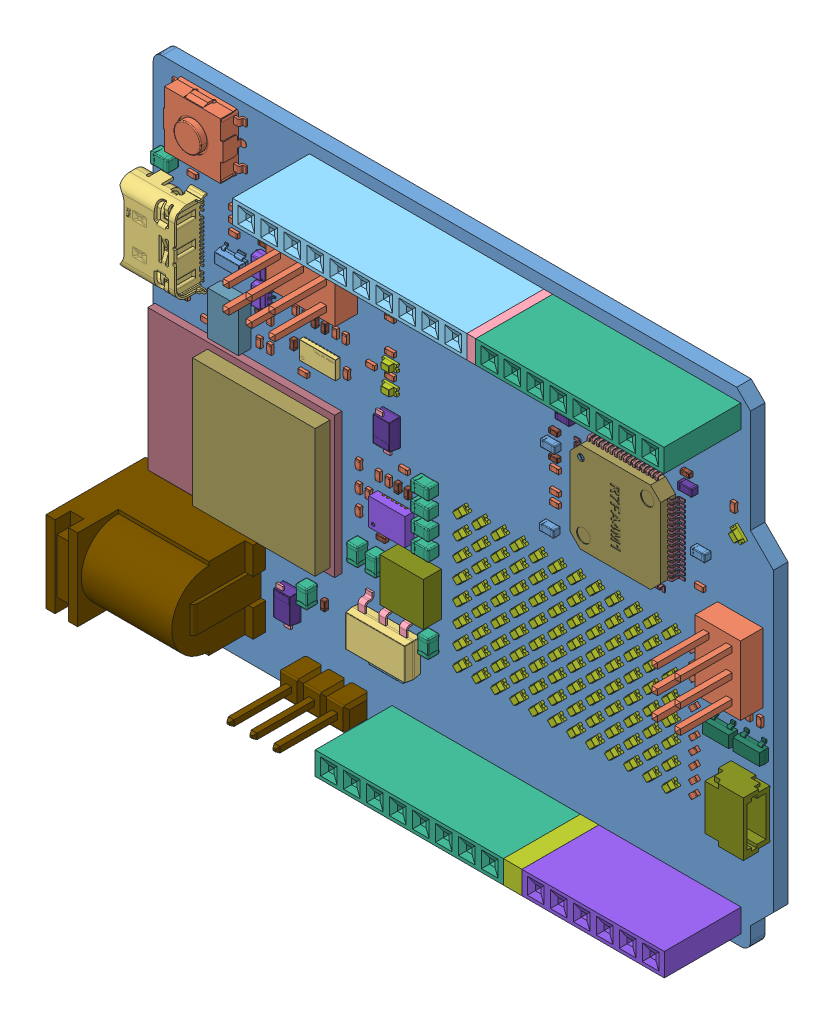
SolidWorks assembly Arduino UnoR4 Wifi PCB(ABX00087), configuration Standard. Lengths in mm.
Overall size (70.54 53.34 14.5).
574 component instances, 44 part files, 0 mates.
Components (placement in the parent):
- PCB(ABX00087).step-1: PCB(ABX00087).step [Standard] at origin size (70.54 53.34 14.5)
  - Board.step-1: Board.step [Standard] at origin size (68.58 53.34 1.61)
    - Open CASCADE STEP translator 7.5 4.1.1.step-1: Open CASCADE STEP translator 7.5 4.1.1.step [Standard] at (0 0 -1.6063) size (68.58 53.34 1.61)
  - R60.step-1: R60.step [Standard] at origin size (1 0.5 0.34)
    - RES-0402.step-1: RES-0402.step [Standard] at (26.4 44.3 0) size (1 0.5 0.34)
  - R59.step-1: R59.step [Standard] at origin size (1 0.5 0.34)
    - RES-0402.step-1: RES-0402.step [Standard] at (26.416 41.021 0) x (-1 0 0) z (0 0 1) size (1 0.5 0.34)
  - R20.step-1: R20.step [Standard] at origin size (1 0.5 0.34)
    - RES-0402.step-1: RES-0402.step [Standard] at (24.29 35.433 0) x (-1 0 0) z (0 0 1) size (1 0.5 0.34)
  - U5.step-1: U5.step [Standard] at origin size (6.71 7 1.8)
    - 6430901664.step-1: 6430901664.step [Standard] at (26.325 10.206 0) x (0 -1 0) z (0 0 1) size (7 6.71 1.8)
      - Body.step-1: Body.step [Standard] at (-1.85 -3.35 0.02) size (3.71 6.71 1.78)
        - Open CASCADE STEP translator 6.8 29.1.1.step-1: Open CASCADE STEP translator 6.8 29.1.1.step [Standard] at origin size (3.71 6.71 1.78)
      - Lead.step-1: Lead.step [Standard] at (-1.85 -2.3 0) x (-1 0 0) z (0 0 1) size (1.65 0.75 1.01)
      - Lead.step-2: Lead.step [Standard] at (-1.85 0 0) x (-1 0 0) z (0 0 1) size (1.65 0.75 1.01)
      - Lead.step-3: Lead.step [Standard] at (-1.85 2.3 0) x (-1 0 0) z (0 0 1) size (1.65 0.75 1.01)
      - Tab.step-1: Tab.step [Standard] at (1.85 0 0) size (1.65 3 1.01)
  - C28.step-1: C28.step [Standard] at origin size (1.25 2 1.25)
    - CAP-0805.step-1: CAP-0805.step [Standard] at (31.0249 12.3561 0) x (0 1 0) z (0 0 1) size (2 1.25 1.25)
  - R58.step-1: R58.step [Standard] at origin size (1 0.5 0.34)
    - RES-0402.step-1: RES-0402.step [Standard] at (16.825 30.966 0) x (-1 0 0) z (0 0 1) size (1 0.5 0.34)
  - R57.step-1: R57.step [Standard] at origin size (1 0.5 0.34)
    - RES-0402.step-1: RES-0402.step [Standard] at (3.625 31.766 0) size (1 0.5 0.34)
  - R16.step-1: R16.step [Standard] at origin size (1.06 1.06 0.34)
    - RES-0402.step-1: RES-0402.step [Standard] at (60.0141 13.5803 0) x (0.707107 0.707107 0) z (0 0 1) size (1 0.5 0.34)
  - R14.step-1: R14.step [Standard] at origin size (1.06 1.06 0.34)
    - RES-0402.step-1: RES-0402.step [Standard] at (60.0141 12.1803 0) x (0.707107 0.707107 0) z (0 0 1) size (1 0.5 0.34)
  - R2.step-1: R2.step [Standard] at origin size (1.06 1.06 0.34)
    - RES-0402.step-1: RES-0402.step [Standard] at (59.9205 26.112 0) x (0.707107 0.707107 0) z (0 0 1) size (1 0.5 0.34)
  - 96.step-1: 96.step [Standard] at origin size (1.7 1.7 0.8)
    - HSMx-190.step-1: HSMx-190.step [Standard] at (57.5124 11.8305 0) x (-0.707107 -0.707107 0) z (0 0 1) size (1.6 0.8 0.8)
  - 95.step-1: 95.step [Standard] at origin size (1.7 1.7 0.8)
    - HSMx-190.step-1: HSMx-190.step [Standard] at (55.4124 11.8305 0) x (-0.707107 -0.707107 0) z (0 0 1) size (1.6 0.8 0.8)
  - 94.step-1: 94.step [Standard] at origin size (1.7 1.7 0.8)
    - HSMx-190.step-1: HSMx-190.step [Standard] at (53.3124 11.8305 0) x (-0.707107 -0.707107 0) z (0 0 1) size (1.6 0.8 0.8)
  - 93.step-1: 93.step [Standard] at origin size (1.7 1.7 0.8)
    - HSMx-190.step-1: HSMx-190.step [Standard] at (51.2124 11.8305 0) x (-0.707107 -0.707107 0) z (0 0 1) size (1.6 0.8 0.8)
  - 92.step-1: 92.step [Standard] at origin size (1.7 1.7 0.8)
    - HSMx-190.step-1: HSMx-190.step [Standard] at (49.1124 11.8305 0) x (-0.707107 -0.707107 0) z (0 0 1) size (1.6 0.8 0.8)
  - 91.step-1: 91.step [Standard] at origin size (1.7 1.7 0.8)
    - HSMx-190.step-1: HSMx-190.step [Standard] at (47.0124 11.8305 0) x (-0.707107 -0.707107 0) z (0 0 1) size (1.6 0.8 0.8)
  - 90.step-1: 90.step [Standard] at origin size (1.7 1.7 0.8)
    - HSMx-190.step-1: HSMx-190.step [Standard] at (44.9124 11.8305 0) x (-0.707107 -0.707107 0) z (0 0 1) size (1.6 0.8 0.8)
  - 89.step-1: 89.step [Standard] at origin size (1.7 1.7 0.8)
    - HSMx-190.step-1: HSMx-190.step [Standard] at (42.8124 11.8305 0) x (-0.707107 -0.707107 0) z (0 0 1) size (1.6 0.8 0.8)
  - 88.step-1: 88.step [Standard] at origin size (1.7 1.7 0.8)
    - HSMx-190.step-1: HSMx-190.step [Standard] at (40.7124 11.8305 0) x (-0.707107 -0.707107 0) z (0 0 1) size (1.6 0.8 0.8)
  - 87.step-1: 87.step [Standard] at origin size (1.7 1.7 0.8)
    - HSMx-190.step-1: HSMx-190.step [Standard] at (38.6124 11.8305 0) x (-0.707107 -0.707107 0) z (0 0 1) size (1.6 0.8 0.8)
  - 86.step-1: 86.step [Standard] at origin size (1.7 1.7 0.8)
    - HSMx-190.step-1: HSMx-190.step [Standard] at (36.5124 11.8305 0) x (-0.707107 -0.707107 0) z (0 0 1) size (1.6 0.8 0.8)
  - 85.step-1: 85.step [Standard] at origin size (1.7 1.7 0.8)
    - HSMx-190.step-1: HSMx-190.step [Standard] at (34.4124 11.8305 0) x (-0.707107 -0.707107 0) z (0 0 1) size (1.6 0.8 0.8)
  - 84.step-1: 84.step [Standard] at origin size (1.7 1.7 0.8)
    - HSMx-190.step-1: HSMx-190.step [Standard] at (57.5124 13.9305 0) x (-0.707107 -0.707107 0) z (0 0 1) size (1.6 0.8 0.8)
  - 83.step-1: 83.step [Standard] at origin size (1.7 1.7 0.8)
    - HSMx-190.step-1: HSMx-190.step [Standard] at (55.4124 13.9305 0) x (-0.707107 -0.707107 0) z (0 0 1) size (1.6 0.8 0.8)
  - 82.step-1: 82.step [Standard] at origin size (1.7 1.7 0.8)
    - HSMx-190.step-1: HSMx-190.step [Standard] at (53.3 13.9182 0) x (-0.707107 -0.707107 0) z (0 0 1) size (1.6 0.8 0.8)
  - 81.step-1: 81.step [Standard] at origin size (1.7 1.7 0.8)
    - HSMx-190.step-1: HSMx-190.step [Standard] at (51.2124 13.9305 0) x (-0.707107 -0.707107 0) z (0 0 1) size (1.6 0.8 0.8)
  - 80.step-1: 80.step [Standard] at origin size (1.7 1.7 0.8)
    - HSMx-190.step-1: HSMx-190.step [Standard] at (49.1124 13.9305 0) x (-0.707107 -0.707107 0) z (0 0 1) size (1.6 0.8 0.8)
  - 79.step-1: 79.step [Standard] at origin size (1.7 1.7 0.8)
    - HSMx-190.step-1: HSMx-190.step [Standard] at (47.0124 13.9305 0) x (-0.707107 -0.707107 0) z (0 0 1) size (1.6 0.8 0.8)
  - 78.step-1: 78.step [Standard] at origin size (1.7 1.7 0.8)
    - HSMx-190.step-1: HSMx-190.step [Standard] at (44.9124 13.9305 0) x (-0.707107 -0.707107 0) z (0 0 1) size (1.6 0.8 0.8)
  - 77.step-1: 77.step [Standard] at origin size (1.7 1.7 0.8)
    - HSMx-190.step-1: HSMx-190.step [Standard] at (42.8124 13.9305 0) x (-0.707107 -0.707107 0) z (0 0 1) size (1.6 0.8 0.8)
  - 76.step-1: 76.step [Standard] at origin size (1.7 1.7 0.8)
    - HSMx-190.step-1: HSMx-190.step [Standard] at (40.7124 13.9305 0) x (-0.707107 -0.707107 0) z (0 0 1) size (1.6 0.8 0.8)
  - 75.step-1: 75.step [Standard] at origin size (1.7 1.7 0.8)
    - HSMx-190.step-1: HSMx-190.step [Standard] at (38.6124 13.9305 0) x (-0.707107 -0.707107 0) z (0 0 1) size (1.6 0.8 0.8)
  - 74.step-1: 74.step [Standard] at origin size (1.7 1.7 0.8)
    - HSMx-190.step-1: HSMx-190.step [Standard] at (36.5124 13.9305 0) x (-0.707107 -0.707107 0) z (0 0 1) size (1.6 0.8 0.8)
  - 73.step-1: 73.step [Standard] at origin size (1.7 1.7 0.8)
    - HSMx-190.step-1: HSMx-190.step [Standard] at (34.4124 13.9305 0) x (-0.707107 -0.707107 0) z (0 0 1) size (1.6 0.8 0.8)
  - 72.step-1: 72.step [Standard] at origin size (1.7 1.7 0.8)
    - HSMx-190.step-1: HSMx-190.step [Standard] at (57.5124 16.0305 0) x (-0.707107 -0.707107 0) z (0 0 1) size (1.6 0.8 0.8)
  - 71.step-1: 71.step [Standard] at origin size (1.7 1.7 0.8)
    - HSMx-190.step-1: HSMx-190.step [Standard] at (55.4124 16.0305 0) x (-0.707107 -0.707107 0) z (0 0 1) size (1.6 0.8 0.8)
  - 70.step-1: 70.step [Standard] at origin size (1.7 1.7 0.8)
    - HSMx-190.step-1: HSMx-190.step [Standard] at (53.3124 16.0305 0) x (-0.707107 -0.707107 0) z (0 0 1) size (1.6 0.8 0.8)
  - 69.step-1: 69.step [Standard] at origin size (1.7 1.7 0.8)
    - HSMx-190.step-1: HSMx-190.step [Standard] at (51.2124 16.0305 0) x (-0.707107 -0.707107 0) z (0 0 1) size (1.6 0.8 0.8)
  - 68.step-1: 68.step [Standard] at origin size (1.7 1.7 0.8)
    - HSMx-190.step-1: HSMx-190.step [Standard] at (49.1124 16.0305 0) x (-0.707107 -0.707107 0) z (0 0 1) size (1.6 0.8 0.8)
  - 67.step-1: 67.step [Standard] at origin size (1.7 1.7 0.8)
    - HSMx-190.step-1: HSMx-190.step [Standard] at (47.0124 16.0305 0) x (-0.707107 -0.707107 0) z (0 0 1) size (1.6 0.8 0.8)
  - 66.step-1: 66.step [Standard] at origin size (1.7 1.7 0.8)
    - HSMx-190.step-1: HSMx-190.step [Standard] at (44.9124 16.0305 0) x (-0.707107 -0.707107 0) z (0 0 1) size (1.6 0.8 0.8)
  - 65.step-1: 65.step [Standard] at origin size (1.7 1.7 0.8)
    - HSMx-190.step-1: HSMx-190.step [Standard] at (42.8124 16.0305 0) x (-0.707107 -0.707107 0) z (0 0 1) size (1.6 0.8 0.8)
  - 64.step-1: 64.step [Standard] at origin size (1.7 1.7 0.8)
    - HSMx-190.step-1: HSMx-190.step [Standard] at (40.7124 16.0305 0) x (-0.707107 -0.707107 0) z (0 0 1) size (1.6 0.8 0.8)
  - 63.step-1: 63.step [Standard] at origin size (1.7 1.7 0.8)
    - HSMx-190.step-1: HSMx-190.step [Standard] at (38.6124 16.0305 0) x (-0.707107 -0.707107 0) z (0 0 1) size (1.6 0.8 0.8)
  - 62.step-1: 62.step [Standard] at origin size (1.7 1.7 0.8)
    - HSMx-190.step-1: HSMx-190.step [Standard] at (36.5124 16.0305 0) x (-0.707107 -0.707107 0) z (0 0 1) size (1.6 0.8 0.8)
  - 61.step-1: 61.step [Standard] at origin size (1.7 1.7 0.8)
    - HSMx-190.step-1: HSMx-190.step [Standard] at (34.412 16.0302 0) x (-0.707107 -0.707107 0) z (0 0 1) size (1.6 0.8 0.8)
  - 60.step-1: 60.step [Standard] at origin size (1.7 1.7 0.8)
    - HSMx-190.step-1: HSMx-190.step [Standard] at (57.5124 18.1305 0) x (-0.707107 -0.707107 0) z (0 0 1) size (1.6 0.8 0.8)
  - 59.step-1: 59.step [Standard] at origin size (1.7 1.7 0.8)
    - HSMx-190.step-1: HSMx-190.step [Standard] at (55.4124 18.1305 0) x (-0.707107 -0.707107 0) z (0 0 1) size (1.6 0.8 0.8)
  - 58.step-1: 58.step [Standard] at origin size (1.7 1.7 0.8)
    - HSMx-190.step-1: HSMx-190.step [Standard] at (53.3124 18.1305 0) x (-0.707107 -0.707107 0) z (0 0 1) size (1.6 0.8 0.8)
  - 57.step-1: 57.step [Standard] at origin size (1.7 1.7 0.8)
    - HSMx-190.step-1: HSMx-190.step [Standard] at (51.2124 18.1305 0) x (-0.707107 -0.707107 0) z (0 0 1) size (1.6 0.8 0.8)
  - 56.step-1: 56.step [Standard] at origin size (1.7 1.7 0.8)
    - HSMx-190.step-1: HSMx-190.step [Standard] at (49.1124 18.1305 0) x (-0.707107 -0.707107 0) z (0 0 1) size (1.6 0.8 0.8)
  - U6.step-1: U6.step [Standard] at origin size (2.1 2.21 1.1)
    - 6430901184.step-1: 6430901184.step [Standard] at (12.525 36.466 0) x (-1 0 0) z (0 0 1) size (2.1 2.21 1.1)
      - Body-1.step-1: Body-1.step [Standard] at (-0.7 -1.1 0) size (1.41 2.21 1.1)
        - Open CASCADE STEP translator 7.5 28.2.1.step-1: Open CASCADE STEP translator 7.5 28.2.1.step [Standard] at origin size (1.41 2.21 1.1)
      - Open CASCADE STEP translator 7.5 28.1.step-1: Open CASCADE STEP translator 7.5 28.1.step [Standard] at (-0.7 -1.1 0.001) size (0.18 0.18 0)
      - Leader.step-1: Leader.step [Standard] at (-0.7 -0.65 0) x (-1 0 0) z (0 0 1) size (0.37 0.2 0.6)
      - Leader.step-2: Leader.step [Standard] at (-0.7 0 0) x (-1 0 0) z (0 0 1) size (0.37 0.2 0.6)
      - Leader.step-3: Leader.step [Standard] at (-0.7 0.65 0) x (-1 0 0) z (0 0 1) size (0.37 0.2 0.6)
      - Leader.step-4: Leader.step [Standard] at (0.7 -0.65 0) size (0.37 0.2 0.6)
      - Leader.step-5: Leader.step [Standard] at (0.7 0 0) size (0.37 0.2 0.6)
      - Leader.step-6: Leader.step [Standard] at (0.7 0.65 0) size (0.37 0.2 0.6)
  - U2.step-1: U2.step [Standard] at origin size (2.1 2.21 1.1)
    - 6430901184.step-1: 6430901184.step [Standard] at (12.525 39.266 0) x (-1 0 0) z (0 0 1) size (2.1 2.21 1.1)
      - Body-1.step-1: Body-1.step [Standard] at (-0.7 -1.1 0) size (1.41 2.21 1.1)
        - Open CASCADE STEP translator 7.5 28.2.1.step-1: Open CASCADE STEP translator 7.5 28.2.1.step [Standard] at origin size (1.41 2.21 1.1)
      - Open CASCADE STEP translator 7.5 28.1.step-1: Open CASCADE STEP translator 7.5 28.1.step [Standard] at (-0.7 -1.1 0.001) size (0.18 0.18 0)
      - Leader.step-1: Leader.step [Standard] at (-0.7 -0.65 0) x (-1 0 0) z (0 0 1) size (0.37 0.2 0.6)
      - Leader.step-2: Leader.step [Standard] at (-0.7 0 0) x (-1 0 0) z (0 0 1) size (0.37 0.2 0.6)
      - Leader.step-3: Leader.step [Standard] at (-0.7 0.65 0) x (-1 0 0) z (0 0 1) size (0.37 0.2 0.6)
      - Leader.step-4: Leader.step [Standard] at (0.7 -0.65 0) size (0.37 0.2 0.6)
      - Leader.step-5: Leader.step [Standard] at (0.7 0 0) size (0.37 0.2 0.6)
      - Leader.step-6: Leader.step [Standard] at (0.7 0.65 0) size (0.37 0.2 0.6)
  - C30.step-1: C30.step [Standard] at origin size (1 0.5 0.5)
    - CAP-0402.step-1: CAP-0402.step [Standard] at (12.525 41.266 0) x (-1 0 0) z (0 0 1) size (1 0.5 0.5)
  - C29.step-1: C29.step [Standard] at origin size (0.5 1 0.5)
    - CAP-0402.step-1: CAP-0402.step [Standard] at (11.925 34.231 0) x (0 1 0) z (0 0 1) size (1 0.5 0.5)
  - R3.step-1: R3.step [Standard] at origin size (0.5 1 0.34)
    - RES-0402.step-1: RES-0402.step [Standard] at (13.466 47.244 0) x (0 -1 0) z (0 0 1) size (1 0.5 0.34)
  - M1.step-1: M1.step [Standard] at origin size (20.65 15.55 2.45)
    - 6428909520.step-1: 6428909520.step [Standard] at (13.625 21.5 0.05) size (13.55 14.15 2.45)
      - Extruded.step-1: Extruded.step [Standard] at origin size (13.55 14.15 2.45)
    - 6428905200.step-1: 6428905200.step [Standard] at (10.575 21.5 0.05) size (20.65 15.55 0.8)
      - Extruded-0.step-1: Extruded-0.step [Standard] at origin size (20.65 15.55 0.8)
  - F1.step-1: F1.step [Standard] at origin size (3.4 4.8 1.4)
    - 6431039776.step-1: 6431039776.step [Standard] at (9.125 32.603 0) size (3.4 4.8 1.4)
      - Extruded-1.step-1: Extruded-1.step [Standard] at origin size (3.4 4.8 1.4)
  - R52.step-1: R52.step [Standard] at origin size (1 0.5 0.34)
    - RES-0402.step-1: RES-0402.step [Standard] at (9.125 42.8599 0) size (1 0.5 0.34)
  - R26.step-1: R26.step [Standard] at origin size (1 0.5 0.34)
    - RES-0402.step-1: RES-0402.step [Standard] at (6.025 30.666 0) x (-1 0 0) z (0 0 1) size (1 0.5 0.34)
  - R12.step-1: R12.step [Standard] at origin size (0.5 1 0.34)
    - RES-0402.step-1: RES-0402.step [Standard] at (67.2698 22.8345 0) x (0 -1 0) z (0 0 1) size (1 0.5 0.34)
  - R11.step-1: R11.step [Standard] at origin size (0.5 1 0.34)
    - RES-0402.step-1: RES-0402.step [Standard] at (66.0698 22.8345 0) x (0 -1 0) z (0 0 1) size (1 0.5 0.34)
  - R10.step-1: R10.step [Standard] at origin size (0.5 1 0.34)
    - RES-0402.step-1: RES-0402.step [Standard] at (63.8698 22.8345 0) x (0 -1 0) z (0 0 1) size (1 0.5 0.34)
  - R9.step-1: R9.step [Standard] at origin size (0.5 1 0.34)
    - RES-0402.step-1: RES-0402.step [Standard] at (62.6698 22.8345 0) x (0 -1 0) z (0 0 1) size (1 0.5 0.34)
  - Q2.step-1: Q2.step [Standard] at origin size (3 2.5 1.1)
    - SOT-23.step-1: SOT-23.step [Standard] at (66.6698 20.0344 0.55) x (1 0 0) z (0 -1 0) size (3 1.1 2.5)
  - Q1.step-1: Q1.step [Standard] at origin size (3 2.5 1.1)
    - SOT-23.step-1: SOT-23.step [Standard] at (63.2698 20.0344 0.55) x (1 0 0) z (0 -1 0) size (3 1.1 2.5)
  - J2.step-1: J2.step [Standard] at origin size (4.95 6 2.96)
    - SM04B-SRSS-TB_RGB12040119.step-1: SM04B-SRSS-TB_RGB12040119.step [Standard] at (64.3195 14.346 -0.28) x (0 1 0) z (1 0 0) size (6 2.96 4.95)
  - R13.step-1: R13.step [Standard] at origin size (1 0.5 0.34)
    - RES-0402.step-1: RES-0402.step [Standard] at (44.646 35.676 0) x (-1 0 0) z (0 0 1) size (1 0.5 0.34)
  - R47.step-1: R47.step [Standard] at origin size (0.5 1 0.34)
    - RES-0402.step-1: RES-0402.step [Standard] at (20.346 36.576 0) x (0 -1 0) z (0 0 1) size (1 0.5 0.34)
  - R48.step-1: R48.step [Standard] at origin size (0.5 1 0.34)
    - RES-0402.step-1: RES-0402.step [Standard] at (21.446 36.576 0) x (0 -1 0) z (0 0 1) size (1 0.5 0.34)
  - R46.step-1: R46.step [Standard] at origin size (0.5 1 0.34)
    - RES-0402.step-1: RES-0402.step [Standard] at (15.946 36.576 0) x (0 -1 0) z (0 0 1) size (1 0.5 0.34)
  - R45.step-1: R45.step [Standard] at origin size (0.5 1 0.34)
    - RES-0402.step-1: RES-0402.step [Standard] at (17.046 36.576 0) x (0 -1 0) z (0 0 1) size (1 0.5 0.34)
  - R31.step-1: R31.step [Standard] at origin size (1.06 1.06 0.34)
    - RES-0402.step-1: RES-0402.step [Standard] at (60.0141 20.5803 0) x (0.707107 0.707107 0) z (0 0 1) size (1 0.5 0.34)
  - 42.step-1: 42.step [Standard] at origin size (1.7 1.7 0.8)
    - HSMx-190.step-1: HSMx-190.step [Standard] at (44.9124 20.2305 0) x (-0.707107 -0.707107 0) z (0 0 1) size (1.6 0.8 0.8)
  - R34.step-1: R34.step [Standard] at origin size (1.06 1.06 0.34)
    - RES-0402.step-1: RES-0402.step [Standard] at (60.0141 24.7803 0) x (0.707107 0.707107 0) z (0 0 1) size (1 0.5 0.34)
  - R33.step-1: R33.step [Standard] at origin size (1.06 1.06 0.34)
    - RES-0402.step-1: RES-0402.step [Standard] at (60.0141 23.3803 0) x (0.707107 0.707107 0) z (0 0 1) size (1 0.5 0.34)
  - R32.step-1: R32.step [Standard] at origin size (1.06 1.06 0.34)
    - RES-0402.step-1: RES-0402.step [Standard] at (60.0141 21.9803 0) x (0.707107 0.707107 0) z (0 0 1) size (1 0.5 0.34)
  - R30.step-1: R30.step [Standard] at origin size (1.06 1.06 0.34)
    - RES-0402.step-1: RES-0402.step [Standard] at (60.0141 19.1803 0) x (0.707107 0.707107 0) z (0 0 1) size (1 0.5 0.34)
  - R29.step-1: R29.step [Standard] at origin size (1.06 1.06 0.34)
    - RES-0402.step-1: RES-0402.step [Standard] at (60.0141 17.7803 0) x (0.707107 0.707107 0) z (0 0 1) size (1 0.5 0.34)
  - R28.step-1: R28.step [Standard] at origin size (1.06 1.06 0.34)
    - RES-0402.step-1: RES-0402.step [Standard] at (60.0141 16.3803 0) x (0.707107 0.707107 0) z (0 0 1) size (1 0.5 0.34)
  - R27.step-1: R27.step [Standard] at origin size (1.06 1.06 0.34)
    - RES-0402.step-1: RES-0402.step [Standard] at (60.0141 14.9803 0) x (0.707107 0.707107 0) z (0 0 1) size (1 0.5 0.34)
  - 54.step-1: 54.step [Standard] at origin size (1.7 1.7 0.8)
    - HSMx-190.step-1: HSMx-190.step [Standard] at (44.9124 18.1305 0) x (-0.707107 -0.707107 0) z (0 0 1) size (1.6 0.8 0.8)
  - 52.step-1: 52.step [Standard] at origin size (1.7 1.7 0.8)
    - HSMx-190.step-1: HSMx-190.step [Standard] at (40.7124 18.1305 0) x (-0.707107 -0.707107 0) z (0 0 1) size (1.6 0.8 0.8)
  - 50.step-1: 50.step [Standard] at origin size (1.7 1.7 0.8)
    - HSMx-190.step-1: HSMx-190.step [Standard] at (36.5124 18.1305 0) x (-0.707107 -0.707107 0) z (0 0 1) size (1.6 0.8 0.8)
  - 48.step-1: 48.step [Standard] at origin size (1.7 1.7 0.8)
    - HSMx-190.step-1: HSMx-190.step [Standard] at (57.5124 20.2305 0) x (-0.707107 -0.707107 0) z (0 0 1) size (1.6 0.8 0.8)
  - 46.step-1: 46.step [Standard] at origin size (1.7 1.7 0.8)
    - HSMx-190.step-1: HSMx-190.step [Standard] at (53.3124 20.2305 0) x (-0.707107 -0.707107 0) z (0 0 1) size (1.6 0.8 0.8)
  - 44.step-1: 44.step [Standard] at origin size (1.7 1.7 0.8)
    - HSMx-190.step-1: HSMx-190.step [Standard] at (49.1124 20.2305 0) x (-0.707107 -0.707107 0) z (0 0 1) size (1.6 0.8 0.8)
  - 55.step-1: 55.step [Standard] at origin size (1.7 1.7 0.8)
    - HSMx-190.step-1: HSMx-190.step [Standard] at (47.0124 18.1305 0) x (-0.707107 -0.707107 0) z (0 0 1) size (1.6 0.8 0.8)
  - 53.step-1: 53.step [Standard] at origin size (1.7 1.7 0.8)
    - HSMx-190.step-1: HSMx-190.step [Standard] at (42.8124 18.1305 0) x (-0.707107 -0.707107 0) z (0 0 1) size (1.6 0.8 0.8)
  - 51.step-1: 51.step [Standard] at origin size (1.7 1.7 0.8)
    - HSMx-190.step-1: HSMx-190.step [Standard] at (38.6124 18.1305 0) x (-0.707107 -0.707107 0) z (0 0 1) size (1.6 0.8 0.8)
  - 49.step-1: 49.step [Standard] at origin size (1.7 1.7 0.8)
    - HSMx-190.step-1: HSMx-190.step [Standard] at (34.4124 18.1305 0) x (-0.707107 -0.707107 0) z (0 0 1) size (1.6 0.8 0.8)
  - 47.step-1: 47.step [Standard] at origin size (1.7 1.7 0.8)
    - HSMx-190.step-1: HSMx-190.step [Standard] at (55.4124 20.2305 0) x (-0.707107 -0.707107 0) z (0 0 1) size (1.6 0.8 0.8)
  - 45.step-1: 45.step [Standard] at origin size (1.7 1.7 0.8)
    - HSMx-190.step-1: HSMx-190.step [Standard] at (51.2124 20.2305 0) x (-0.707107 -0.707107 0) z (0 0 1) size (1.6 0.8 0.8)
  - 43.step-1: 43.step [Standard] at origin size (1.7 1.7 0.8)
    - HSMx-190.step-1: HSMx-190.step [Standard] at (47.0124 20.2305 0) x (-0.707107 -0.707107 0) z (0 0 1) size (1.6 0.8 0.8)
  - 40.step-1: 40.step [Standard] at origin size (1.7 1.7 0.8)
    - HSMx-190.step-1: HSMx-190.step [Standard] at (40.7124 20.2305 0) x (-0.707107 -0.707107 0) z (0 0 1) size (1.6 0.8 0.8)
  - 38.step-1: 38.step [Standard] at origin size (1.7 1.7 0.8)
    - HSMx-190.step-1: HSMx-190.step [Standard] at (36.5124 20.2305 0) x (-0.707107 -0.707107 0) z (0 0 1) size (1.6 0.8 0.8)
  - 36.step-1: 36.step [Standard] at origin size (1.7 1.7 0.8)
    - HSMx-190.step-1: HSMx-190.step [Standard] at (57.5124 22.3305 0) x (-0.707107 -0.707107 0) z (0 0 1) size (1.6 0.8 0.8)
  - 34.step-1: 34.step [Standard] at origin size (1.7 1.7 0.8)
    - HSMx-190.step-1: HSMx-190.step [Standard] at (53.3124 22.3305 0) x (-0.707107 -0.707107 0) z (0 0 1) size (1.6 0.8 0.8)
  - 32.step-1: 32.step [Standard] at origin size (1.7 1.7 0.8)
    - HSMx-190.step-1: HSMx-190.step [Standard] at (49.1124 22.3305 0) x (-0.707107 -0.707107 0) z (0 0 1) size (1.6 0.8 0.8)
  - 41.step-1: 41.step [Standard] at origin size (1.7 1.7 0.8)
    - HSMx-190.step-1: HSMx-190.step [Standard] at (42.8124 20.2305 0) x (-0.707107 -0.707107 0) z (0 0 1) size (1.6 0.8 0.8)
  - 39.step-1: 39.step [Standard] at origin size (1.7 1.7 0.8)
    - HSMx-190.step-1: HSMx-190.step [Standard] at (38.6124 20.2305 0) x (-0.707107 -0.707107 0) z (0 0 1) size (1.6 0.8 0.8)
  - 37.step-1: 37.step [Standard] at origin size (1.7 1.7 0.8)
    - HSMx-190.step-1: HSMx-190.step [Standard] at (34.4124 20.2305 0) x (-0.707107 -0.707107 0) z (0 0 1) size (1.6 0.8 0.8)
  - 35.step-1: 35.step [Standard] at origin size (1.7 1.7 0.8)
    - HSMx-190.step-1: HSMx-190.step [Standard] at (55.4124 22.3305 0) x (-0.707107 -0.707107 0) z (0 0 1) size (1.6 0.8 0.8)
  - 33.step-1: 33.step [Standard] at origin size (1.7 1.7 0.8)
    - HSMx-190.step-1: HSMx-190.step [Standard] at (51.2124 22.3305 0) x (-0.707107 -0.707107 0) z (0 0 1) size (1.6 0.8 0.8)
  - 31.step-1: 31.step [Standard] at origin size (1.7 1.7 0.8)
    - HSMx-190.step-1: HSMx-190.step [Standard] at (47.0124 22.3305 0) x (-0.707107 -0.707107 0) z (0 0 1) size (1.6 0.8 0.8)
  - 30.step-1: 30.step [Standard] at origin size (1.7 1.7 0.8)
    - HSMx-190.step-1: HSMx-190.step [Standard] at (44.9124 22.3305 0) x (-0.707107 -0.707107 0) z (0 0 1) size (1.6 0.8 0.8)
  - 28.step-1: 28.step [Standard] at origin size (1.7 1.7 0.8)
    - HSMx-190.step-1: HSMx-190.step [Standard] at (40.7124 22.3305 0) x (-0.707107 -0.707107 0) z (0 0 1) size (1.6 0.8 0.8)
  - 26.step-1: 26.step [Standard] at origin size (1.7 1.7 0.8)
    - HSMx-190.step-1: HSMx-190.step [Standard] at (36.5124 22.3305 0) x (-0.707107 -0.707107 0) z (0 0 1) size (1.6 0.8 0.8)
  - 24.step-1: 24.step [Standard] at origin size (1.7 1.7 0.8)
    - HSMx-190.step-1: HSMx-190.step [Standard] at (57.5124 24.4305 0) x (-0.707107 -0.707107 0) z (0 0 1) size (1.6 0.8 0.8)
  - 22.step-1: 22.step [Standard] at origin size (1.7 1.7 0.8)
    - HSMx-190.step-1: HSMx-190.step [Standard] at (53.3124 24.4305 0) x (-0.707107 -0.707107 0) z (0 0 1) size (1.6 0.8 0.8)
  - 29.step-1: 29.step [Standard] at origin size (1.7 1.7 0.8)
    - HSMx-190.step-1: HSMx-190.step [Standard] at (42.8124 22.3305 0) x (-0.707107 -0.707107 0) z (0 0 1) size (1.6 0.8 0.8)
  - 27.step-1: 27.step [Standard] at origin size (1.7 1.7 0.8)
    - HSMx-190.step-1: HSMx-190.step [Standard] at (38.6124 22.3305 0) x (-0.707107 -0.707107 0) z (0 0 1) size (1.6 0.8 0.8)
  - 25.step-1: 25.step [Standard] at origin size (1.7 1.7 0.8)
    - HSMx-190.step-1: HSMx-190.step [Standard] at (34.4124 22.3305 0) x (-0.707107 -0.707107 0) z (0 0 1) size (1.6 0.8 0.8)
  - 23.step-1: 23.step [Standard] at origin size (1.7 1.7 0.8)
    - HSMx-190.step-1: HSMx-190.step [Standard] at (55.4124 24.4305 0) x (-0.707107 -0.707107 0) z (0 0 1) size (1.6 0.8 0.8)
  - 21.step-1: 21.step [Standard] at origin size (1.7 1.7 0.8)
    - HSMx-190.step-1: HSMx-190.step [Standard] at (51.2124 24.4305 0) x (-0.707107 -0.707107 0) z (0 0 1) size (1.6 0.8 0.8)
  - 20.step-1: 20.step [Standard] at origin size (1.7 1.7 0.8)
    - HSMx-190.step-1: HSMx-190.step [Standard] at (49.1124 24.4305 0) x (-0.707107 -0.707107 0) z (0 0 1) size (1.6 0.8 0.8)
  - 18.step-1: 18.step [Standard] at origin size (1.7 1.7 0.8)
    - HSMx-190.step-1: HSMx-190.step [Standard] at (44.9124 24.4305 0) x (-0.707107 -0.707107 0) z (0 0 1) size (1.6 0.8 0.8)
  - 16.step-1: 16.step [Standard] at origin size (1.7 1.7 0.8)
    - HSMx-190.step-1: HSMx-190.step [Standard] at (40.7124 24.4305 0) x (-0.707107 -0.707107 0) z (0 0 1) size (1.6 0.8 0.8)
  - 14.step-1: 14.step [Standard] at origin size (1.7 1.7 0.8)
    - HSMx-190.step-1: HSMx-190.step [Standard] at (36.5124 24.4305 0) x (-0.707107 -0.707107 0) z (0 0 1) size (1.6 0.8 0.8)
  - 19.step-1: 19.step [Standard] at origin size (1.7 1.7 0.8)
    - HSMx-190.step-1: HSMx-190.step [Standard] at (47.0124 24.4305 0) x (-0.707107 -0.707107 0) z (0 0 1) size (1.6 0.8 0.8)
  - 17.step-1: 17.step [Standard] at origin size (1.7 1.7 0.8)
    - HSMx-190.step-1: HSMx-190.step [Standard] at (42.8124 24.4305 0) x (-0.707107 -0.707107 0) z (0 0 1) size (1.6 0.8 0.8)
  - 15.step-1: 15.step [Standard] at origin size (1.7 1.7 0.8)
    - HSMx-190.step-1: HSMx-190.step [Standard] at (38.6124 24.4305 0) x (-0.707107 -0.707107 0) z (0 0 1) size (1.6 0.8 0.8)
  - 13.step-1: 13.step [Standard] at origin size (1.7 1.7 0.8)
    - HSMx-190.step-1: HSMx-190.step [Standard] at (34.4124 24.4305 0) x (-0.707107 -0.707107 0) z (0 0 1) size (1.6 0.8 0.8)
  - 12.step-1: 12.step [Standard] at origin size (1.7 1.7 0.8)
    - HSMx-190.step-1: HSMx-190.step [Standard] at (57.5124 26.5305 0) x (-0.707107 -0.707107 0) z (0 0 1) size (1.6 0.8 0.8)
  - 10.step-1: 10.step [Standard] at origin size (1.7 1.7 0.8)
    - HSMx-190.step-1: HSMx-190.step [Standard] at (53.3124 26.5305 0) x (-0.707107 -0.707107 0) z (0 0 1) size (1.6 0.8 0.8)
  - 8.step-1: 8.step [Standard] at origin size (1.7 1.7 0.8)
    - HSMx-190.step-1: HSMx-190.step [Standard] at (49.1124 26.5305 0) x (-0.707107 -0.707107 0) z (0 0 1) size (1.6 0.8 0.8)
  - 11.step-1: 11.step [Standard] at origin size (1.7 1.7 0.8)
    - HSMx-190.step-1: HSMx-190.step [Standard] at (55.4124 26.5305 0) x (-0.707107 -0.707107 0) z (0 0 1) size (1.6 0.8 0.8)
  - 9.step-1: 9.step [Standard] at origin size (1.7 1.7 0.8)
    - HSMx-190.step-1: HSMx-190.step [Standard] at (51.2124 26.5305 0) x (-0.707107 -0.707107 0) z (0 0 1) size (1.6 0.8 0.8)
  - 7.step-1: 7.step [Standard] at origin size (1.7 1.7 0.8)
    - HSMx-190.step-1: HSMx-190.step [Standard] at (47.0124 26.5305 0) x (-0.707107 -0.707107 0) z (0 0 1) size (1.6 0.8 0.8)
  - 6.step-1: 6.step [Standard] at origin size (1.7 1.7 0.8)
    - HSMx-190.step-1: HSMx-190.step [Standard] at (44.9124 26.5305 0) x (-0.707107 -0.707107 0) z (0 0 1) size (1.6 0.8 0.8)
  - 4.step-1: 4.step [Standard] at origin size (1.7 1.7 0.8)
    - HSMx-190.step-1: HSMx-190.step [Standard] at (40.7124 26.5305 0) x (-0.707107 -0.707107 0) z (0 0 1) size (1.6 0.8 0.8)
  - 5.step-1: 5.step [Standard] at origin size (1.7 1.7 0.8)
    - HSMx-190.step-1: HSMx-190.step [Standard] at (42.8124 26.5305 0) x (-0.707107 -0.707107 0) z (0 0 1) size (1.6 0.8 0.8)
  - 3.step-1: 3.step [Standard] at origin size (1.7 1.7 0.8)
    - HSMx-190.step-1: HSMx-190.step [Standard] at (38.6124 26.5305 0) x (-0.707107 -0.707107 0) z (0 0 1) size (1.6 0.8 0.8)
  - 2.step-1: 2.step [Standard] at origin size (1.7 1.7 0.8)
    - HSMx-190.step-1: HSMx-190.step [Standard] at (36.5124 26.5305 0) x (-0.707107 -0.707107 0) z (0 0 1) size (1.6 0.8 0.8)
  - 1.step-1: 1.step [Standard] at origin size (1.7 1.7 0.8)
    - HSMx-190.step-1: HSMx-190.step [Standard] at (34.4124 26.5305 0) x (-0.707107 -0.707107 0) z (0 0 1) size (1.6 0.8 0.8)
  - R35.step-1: R35.step [Standard] at origin size (0.5 1 0.34)
    - RES-0402.step-1: RES-0402.step [Standard] at (22.925 20.8 0) x (0 1 0) z (0 0 1) size (1 0.5 0.34)
  - Q3.step-1: Q3.step [Standard] at origin size (3 2.5 1.1)
    - SOT-23.step-1: SOT-23.step [Standard] at (12.5251 44.0661 0.55) x (-1 0 0) z (0 1 0) size (3 1.1 2.5)
  - D1.step-1: D1.step [Standard] at origin size (2.01 3.7 1.2)
    - SOD123FL.step-1: SOD123FL.step [Standard] at (13.395 12.306 0) x (0 -1 0) z (0 0 1) size (3.7 2 1.2)
      - 8279795424.step-1: 8279795424.step [Standard] at (4 2 0) size (3.7 2 1.2)
        - Body-2.step-1: Body-2.step [Standard] at (-1.5 -1 0) size (3 2 1.2)
          - Open CASCADE STEP translator 7.5 15.1.1.step-1: Open CASCADE STEP translator 7.5 15.1.1.step [Standard] at origin size (3 2 1.2)
        - Lead.step-1: Lead.step [Standard] at (-1.85 -0.425 0) size (1.65 0.75 1.01)
        - Lead.step-2: Lead.step [Standard] at (1.85 0.425 0) x (-1 0 0) z (0 0 1) size (1.65 0.75 1.01)
  - R42.step-1: R42.step [Standard] at origin size (0.5 1 0.34)
    - RES-0402.step-1: RES-0402.step [Standard] at (24.025 23 0) x (0 -1 0) z (0 0 1) size (1 0.5 0.34)
  - R6.step-1: R6.step [Standard] at origin size (0.5 1 0.34)
    - RES-0402.step-1: RES-0402.step [Standard] at (44.1148 41.903 0) x (0 -1 0) z (0 0 1) size (1 0.5 0.34)
  - JOFF.step-1: JOFF.step [Standard] at origin size (7.62 2.54 12.7)
    - pin4.step-1: pin4.step [Standard] at (22.86 2.54 0) size (2.54 2.54 12.7)
    - pin4.step-2: pin4.step [Standard] at (20.32 2.54 0) size (2.54 2.54 12.7)
    - pin4.step-3: pin4.step [Standard] at (17.78 2.54 0) size (2.54 2.54 12.7)
  - C5.step-1: C5.step [Standard] at origin size (1.6 0.8 0.8)
    - CAP-0603.step-1: CAP-0603.step [Standard] at (44.246 29.876 0) size (1.6 0.8 0.8)
  - C18.step-1: C18.step [Standard] at origin size (2 1.25 1.25)
    - CAP-0805.step-1: CAP-0805.step [Standard] at (30.6449 27.1464 0) x (-1 0 0) z (0 0 1) size (2 1.25 1.25)
  - C17.step-1: C17.step [Standard] at origin size (2 1.25 1.25)
    - CAP-0805.step-1: CAP-0805.step [Standard] at (30.6449 25.1964 0) x (-1 0 0) z (0 0 1) size (2 1.25 1.25)
  - J6.step-1: J6.step [Standard] at origin size (7.62 5.04 11.5)
    - 2x3 Header.step-1: 2x3 Header.step [Standard] at (14.9861 39.4239 0) x (0 1 0) z (1 0 0) size (5.04 11.5 7.62)
  - C10.step-1: C10.step [Standard] at origin size (1.25 2 1.25)
    - CAP-0805.step-1: CAP-0805.step [Standard] at (17.5899 10.4061 0) x (0 1 0) z (0 0 1) size (2 1.25 1.25)
  - U4.step-1: U4.step [Standard] at origin size (4 2 0.55)
    - IC_Texas_Instruments_TXB0108DQSR_eec.step-1: IC_Texas_Instruments_TXB0108DQSR_eec.step [Standard] at (13.565 34.6878 0.3) x (1 0 0) z (0 0 1) size (4 2 0.55)
      - Part15.step-1: Part15.step [Standard] at (5.131 -1.3893 -0.25) size (4 2 0.5)
      - Part16.step-1: Part16.step [Standard] at (3.731 -2.1143 -0.3) size (0.2 0.55 0.1)
      - Part16.step-2: Part16.step [Standard] at (4.131 -2.1143 -0.3) size (0.2 0.55 0.1)
      - Part16.step-3: Part16.step [Standard] at (4.531 -2.1143 -0.3) size (0.2 0.55 0.1)
      - Part16.step-4: Part16.step [Standard] at (4.931 -2.1143 -0.3) size (0.2 0.55 0.1)
